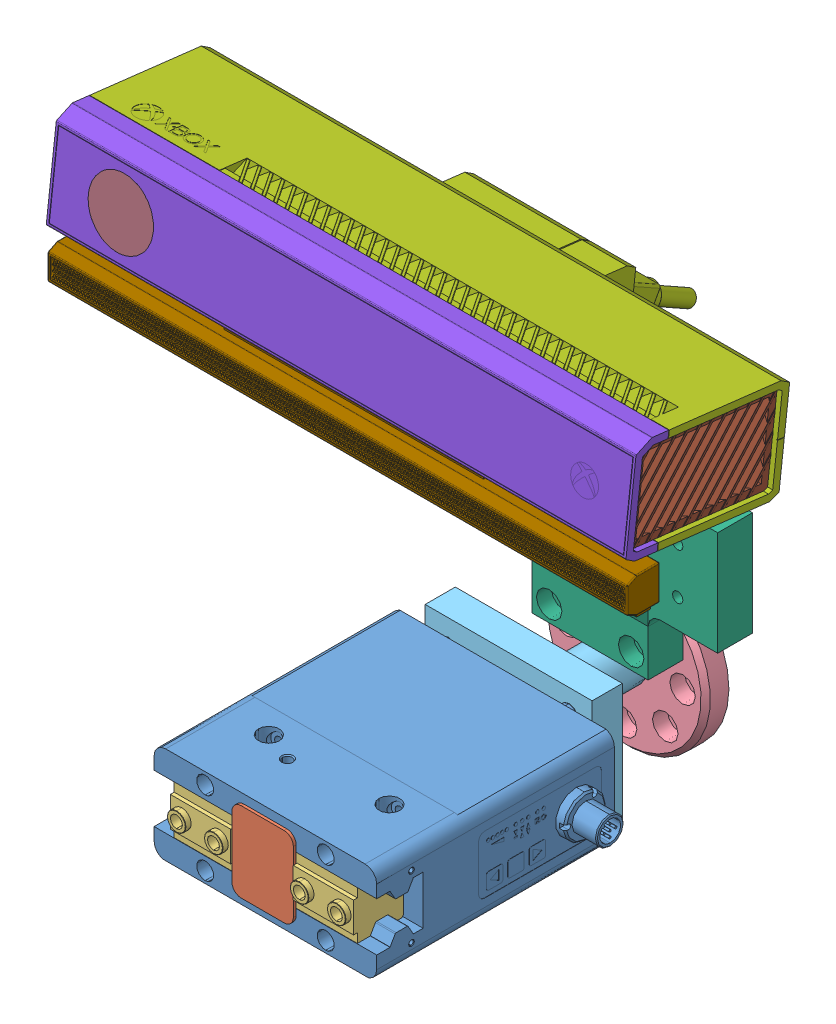
SolidWorks assembly Assem2, configuration Default. Lengths in mm.
Overall size (250 236.61 168.8).
18 component instances, 14 part files, 6 mates.
Components (placement in the parent):
- Gripper and mating plate-1: Gripper and mating plate [Default] at (39.1591 97.0842 110.2166) x (-1 0 0) z (0 1 0) size (110.5 168.8 70.6)
  - _GEP5008IL_00_A_zylinder_1_2-1: _GEP5008IL_00_A_zylinder_1_2 [Default] at origin size (110.5 104.9 42)
  - _GEP5008IL_00_A_deckel_4-1: _GEP5008IL_00_A_deckel_4 [Default] at origin size (26.5 1.2 34.5)
  - _GPP5008NC_00_A1_backen_6-1: _GPP5008NC_00_A1_backen_6 [Default] at (0.5 37 0) size (39 23.9 21)
  - _GPP5008NC_00_A1_backen_6-2: _GPP5008NC_00_A1_backen_6 [Default] at (-0.5 37 0) x (-1 0 0) z (0 0 -1) size (39 23.9 21)
  - Assembly flange-1: Assembly flange [Default] at (45.6292 -41.3631 -11.3851) x (0.999966 0 0.008259) z (0 -1 0) size (72.43 70 60)
    - IIWA Flange-1: IIWA Flange [Default] at (-45.5337 11.7616 11.0369) size (70 70 10)
    - Zimmer GEP5008N bracket-1: Zimmer GEP5008N bracket [Default] at (-45.5337 11.7616 -23.9631) x (-0.999966 0.008259 0) z (0 0 1) size (72 52 50)
- Print bracket-1: Print bracket [Default] at (64.308 244.1982 115.0534) x (0 0 -1) z (0 1 0) size (100 80 125)
- AS1-1: AS1 [Default] at (39.308 234.4072 140.8166) x (-1 0 0) z (0 1 0) size (250 121.83 65.49)
  - 1-1: 1 [Default] at (-125 41.8074 21.2837) x (0 0.993094 0.117321) z (1 0 0) size (114.6 50.3 250)
  - 2-1: 2 [Default] at (-125 28.1027 19.6646) x (0 0.993094 0.117321) z (1 0 0) size (13.8 43 250)
  - 3-1: 3 [Default] at origin size (250 82 32.5)
  - 4-1: 4 [Default] at (120 -21.7062 17.6613) x (0 0.993094 0.117321) z (1 0 0) size (60.5 37 3)
  - 5-1: 5 [Default] at (-120 -21.7062 17.6613) x (0 0.993094 0.117321) z (1 0 0) size (60.5 37 3)
  - 6-1: 6 [Default] at (0 -32.2685 30.3556) x (1 0 0) z (0 -0.993094 -0.117321) size (44 36 8)
  - 7-1: 7 [Default] at (95 36.4213 41.3048) x (-1 0 0) z (0 0.993094 0.117321) size (28 28 3)
  - 8-1: 8 [Default] at (95 31.9524 40.7769) x (-1 0 0) z (0 0.993094 0.117321) size (12 12 4)
Mates (geometry in assembly coordinates):
- Coincident1: coincident aligned: circle of Gripper and mating plate-1/Assembly flange-1/IIWA Flange-1; cylinder of Print bracket-1 through (21.628 114.9072 72.8166) axis (0 0 1) radius 3.3
- Coincident2: coincident anti-aligned: plane of Gripper and mating plate-1/Assembly flange-1/IIWA Flange-1 through (39.1591 97.0842 57.8166) normal (0 0 1); plane of Print bracket-1 through (14.308 232.9072 57.8166) normal (0 0 -1)
- Parallel2: parallel aligned: plane of Gripper and mating plate-1/_GEP5008IL_00_A_zylinder_1_2-1 through (87.1591 81.0842 212.7166) normal (1 0 0); plane of Print bracket-1 through (64.308 244.1982 115.0534) normal (1 0 0)
- Concentric3: concentric: cylinder of Print bracket-1 through (39.308 212.9072 149.8166) axis (0 -1 0) radius 2.75; cylinder of AS1-1/3-1 through (39.308 234.4072 149.8166) axis (0 -1 0) radius 2.5527
- Coincident5: coincident: plane of Print bracket-1 through (14.308 232.9072 157.8166) normal (0 1 0); plane of AS1-1/3-1 through (39.308 232.9072 140.8166) normal (0 -1 0)
- Parallel3: parallel aligned: plane of Print bracket-1 through (14.308 244.1982 115.0534) normal (-1 0 0); plane of AS1-1/1-1 through (-85.692 255.6909 182.624) normal (-1 0 0)
